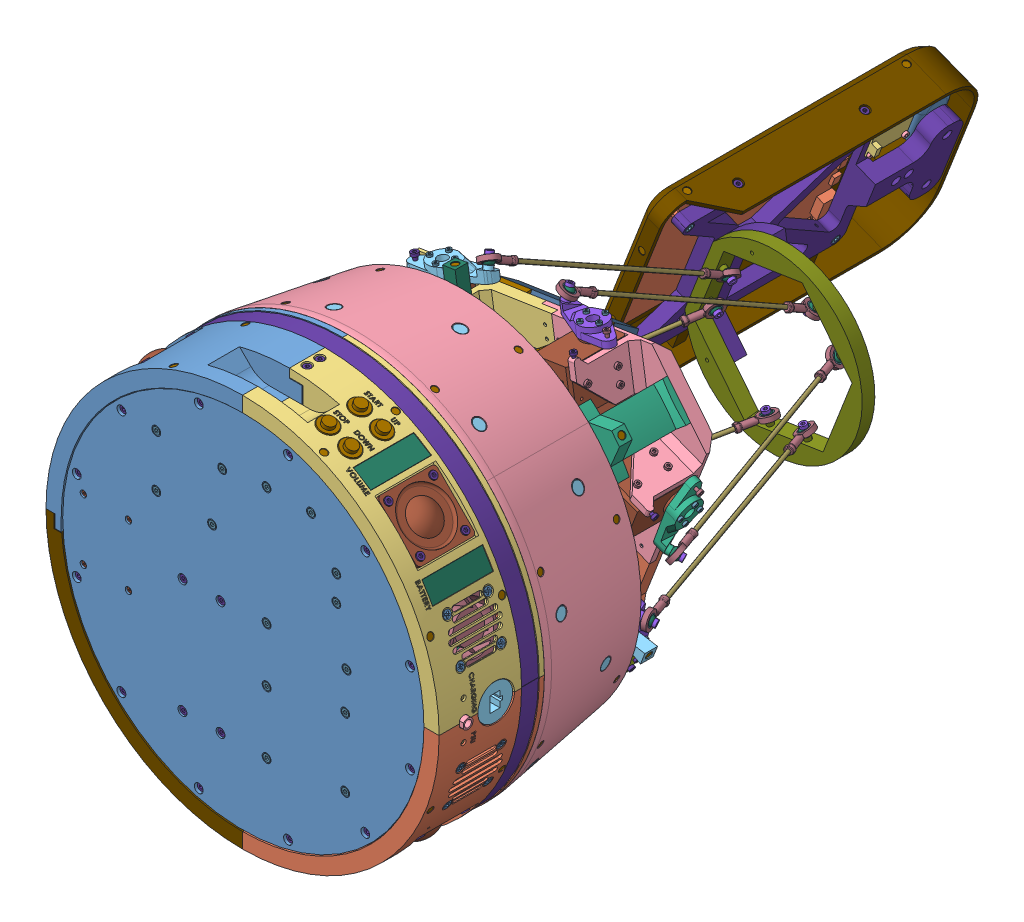
SolidWorks assembly robot orin, configuration Défaut. Lengths in mm.
Overall size (438.41 438.41 602.06).
668 component instances, 95 part files, 23 mates.
Components (placement in the parent):
- base-1: base [Défaut] at (-67.3784 29.2661 438.4062) size (438.41 438.41 173)
  - base disk-1: base disk [Défaut] at (36.9194 20.0613 317) size (285 285 66.55)
    - base disk-1: base disk [Défaut] at (-39.9498 -9.3034 266.18) size (285 285 6.35)
    - Adafruit MAX9744-1: Adafruit MAX9744 [Défaut] at (-148.3839 -9.3034 256.18) x (0 1 0) z (0 0 -1) size (56.74 43.64 13.6)
    - Adafruit MAX9744-2: Adafruit MAX9744 [Défaut] at (-148.3839 -9.3034 239.58) x (0 1 0) z (0 0 -1) size (56.74 43.64 13.6)
    - Battery charger RRC-PMM240-1: Battery charger RRC-PMM240 [Défaut] at (-52.8471 67.1868 256.18) x (0 -1 0) z (0 0 -1) size (57 70 12)
    - battery holder-1: battery holder [Défaut] at (-92.9498 0.6966 266.18) x (0 -1 0) z (1 0 0) size (115 36.2 40)
    - Battery RRC2054-2-1: Battery RRC2054-2 [Défaut] at (-82.3791 -10.7125 233.18) x (0 1 0) z (0 0 1) size (151 78 23)
    - ground loop noise isolator-1: ground loop noise isolator [Défaut] at (-105.1098 -100.3034 233.18) x (0 -1 0) z (1 0 0) size (20 20 60)
    - ground loop noise isolator-2: ground loop noise isolator [Défaut] at (-45.1098 -80.3034 233.18) x (0 0 1) z (-1 0 0) size (20 20 60)
    - psu control-1: psu control [Défaut] at (-25.1498 95.1966 256.18) x (0 -1 0) z (0 0 -1) size (100 70 16.5)
    - buck boost-1: buck boost [Défaut] at (-25.6498 -27.3034 256.18) x (0 -1 0) z (0 0 -1) size (80 70 23.6)
    - buck boost-2: buck boost [Défaut] at (-25.6498 -27.3034 229.58) x (0 -1 0) z (0 0 -1) size (80 70 23.6)
    - 732-12936-ND-1: 732-12936-ND [Défaut] at (-166.1639 14.8266 254.58) x (-0.923728 -0.383049 0) z (0 0 -1) size (4.6 4.17 20)
    - 732-12936-ND-2: 732-12936-ND [Défaut] at (-166.1639 -33.4334 254.58) x (-0.923728 -0.383049 0) z (0 0 -1) size (4.6 4.17 20)
    - 732-12936-ND-3: 732-12936-ND [Défaut] at (-130.6039 -33.4334 254.58) x (-0.923728 -0.383049 0) z (0 0 -1) size (4.6 4.17 20)
    - 732-12936-ND-4: 732-12936-ND [Défaut] at (-130.6039 14.8266 254.58) x (-0.923728 -0.383049 0) z (0 0 -1) size (4.6 4.17 20)
    - 732-12918-ND-1: 732-12918-ND [Défaut] at (-166.1639 14.8266 266.18) x (-0.923728 -0.383049 0) z (0 0 -1) size (4.6 4.17 15)
    - 732-12918-ND-2: 732-12918-ND [Défaut] at (-130.6039 14.8266 266.18) x (-0.923728 -0.383049 0) z (0 0 -1) size (4.6 4.17 15)
    - 732-12918-ND-3: 732-12918-ND [Défaut] at (-130.6039 -33.4334 266.18) x (-0.923728 -0.383049 0) z (0 0 -1) size (4.6 4.17 15)
    - 732-12918-ND-4: 732-12918-ND [Défaut] at (-166.1639 -33.4334 266.18) x (-0.923728 -0.383049 0) z (0 0 -1) size (4.6 4.17 15)
    - M2x8mm socket-6: M2x8mm socket [Défaut] at (-166.1639 -33.4334 262.03) x (-1 0 0) z (0 0 1) size (3.8 3.8 9.6)
    - M2x8mm socket-5: M2x8mm socket [Défaut] at (-130.6039 -33.4334 262.03) x (-1 0 0) z (0 0 1) size (3.8 3.8 9.6)
    - M2x8mm socket-3: M2x8mm socket [Défaut] at (-166.1639 14.8266 262.03) size (3.8 3.8 9.6)
    - M2x8mm socket-4: M2x8mm socket [Défaut] at (-130.6039 14.8266 262.03) x (-1 0 0) z (0 0 1) size (3.8 3.8 9.6)
    - M2 nut-1: M2 nut [Défaut] at (-166.1639 14.8266 237.98) x (-0.923728 -0.383049 0) z (0 0 -1) size (4.62 4 1.6)
    - M2 nut-2: M2 nut [Défaut] at (-166.1639 -33.4334 237.98) x (-0.923728 -0.383049 0) z (0 0 -1) size (4.62 4 1.6)
    - M2 nut-3: M2 nut [Défaut] at (-130.6039 -33.4334 237.98) x (-0.923728 -0.383049 0) z (0 0 -1) size (4.62 4 1.6)
    - M2 nut-4: M2 nut [Défaut] at (-130.6039 14.8266 237.98) x (-0.923728 -0.383049 0) z (0 0 -1) size (4.62 4 1.6)
    - 36-24337-ND-1: 36-24337-ND [Défaut] at (-108.6498 86.6966 266.18) x (-0.923728 -0.383049 0) z (0 0 -1) size (5.77 5 18)
    - 36-24337-ND-2: 36-24337-ND [Défaut] at (-108.6498 45.6966 266.18) x (-0.923728 -0.383049 0) z (0 0 -1) size (5.77 5 18)
    - 36-24337-ND-3: 36-24337-ND [Défaut] at (-64.6498 44.6966 266.18) x (-0.923728 -0.383049 0) z (0 0 -1) size (5.77 5 18)
    - 36-24337-ND-4: 36-24337-ND [Défaut] at (-56.6498 86.6966 266.18) x (-0.923728 -0.383049 0) z (0 0 -1) size (5.77 5 18)
    - M3x5mm socket-1: M3x5mm socket [Défaut] at (-108.6498 86.6966 264.53) x (-1 0 0) z (0 0 1) size (5.5 5.5 8)
    - M3x5mm socket-2: M3x5mm socket [Défaut] at (-108.6498 45.6966 264.53) x (-1 0 0) z (0 0 1) size (5.5 5.5 8)
    - M3x5mm socket-3: M3x5mm socket [Défaut] at (-64.6498 44.6966 264.53) x (-1 0 0) z (0 0 1) size (5.5 5.5 8)
    - M3x5mm socket-4: M3x5mm socket [Défaut] at (-56.6498 86.6966 264.53) x (-1 0 0) z (0 0 1) size (5.5 5.5 8)
    - M3 nut-1: M3 nut [Défaut] at (-108.6498 86.6966 254.18) x (-0.923728 -0.383049 0) z (0 0 -1) size (6.35 5.5 2.4)
    - M3 nut-2: M3 nut [Défaut] at (-108.6498 45.6966 254.18) x (-0.923728 -0.383049 0) z (0 0 -1) size (6.35 5.5 2.4)
    - M3 nut-3: M3 nut [Défaut] at (-64.6498 44.6966 254.18) x (-0.923728 -0.383049 0) z (0 0 -1) size (6.35 5.5 2.4)
    - M3 nut-4: M3 nut [Défaut] at (-56.6498 86.6966 254.18) x (-0.923728 -0.383049 0) z (0 0 -1) size (6.35 5.5 2.4)
    - 36-24337-ND-5: 36-24337-ND [Défaut] at (-21.6498 91.6966 266.18) x (-0.923728 -0.383049 0) z (0 0 -1) size (5.77 5 18)
    - 36-24337-ND-6: 36-24337-ND [Défaut] at (-21.6498 -1.3034 266.18) x (1 0 0) z (0 0 -1) size (5.77 5 18)
    - 36-24337-ND-7: 36-24337-ND [Défaut] at (13.3502 91.6966 266.18) x (0.923728 0.383049 0) z (0 0 -1) size (5.77 5 18)
    - 36-24337-ND-8: 36-24337-ND [Défaut] at (41.3502 -1.3034 266.18) x (-1 0 0) z (0 0 -1) size (5.77 5 18)
    - M3 nut-5: M3 nut [Défaut] at (-21.6498 91.6966 256.98) x (-1 0 0) z (0 0 -1) size (6.35 5.5 2.4)
    - M3 nut-6: M3 nut [Défaut] at (13.3502 91.6966 252.18) x (-1 0 0) z (0 0 1) size (6.35 5.5 2.4)
    - M3 nut-7: M3 nut [Défaut] at (-21.6498 -1.3034 252.18) x (-1 0 0) z (0 0 1) size (6.35 5.5 2.4)
    - M3 nut-8: M3 nut [Défaut] at (41.3502 -1.3034 252.18) size (6.35 5.5 2.4)
    - 36-24337-ND-9: 36-24337-ND [Défaut] at (-21.6498 -44.3034 266.18) x (-0.923728 -0.383049 0) z (0 0 -1) size (5.77 5 18)
    - 36-24337-ND-10: 36-24337-ND [Défaut] at (-21.6498 -93.3034 266.18) x (-0.923728 -0.383049 0) z (0 0 -1) size (5.77 5 18)
    - 36-24337-ND-11: 36-24337-ND [Défaut] at (40.3502 -85.3034 266.18) x (-0.923728 -0.383049 0) z (0 0 -1) size (5.77 5 18)
    - 36-24337-ND-12: 36-24337-ND [Défaut] at (40.3502 -31.3034 266.18) x (-0.923728 -0.383049 0) z (0 0 -1) size (5.77 5 18)
    - 36-24342-ND-1: 36-24342-ND [Défaut] at (-21.6498 -44.3034 254.58) x (1 0 0) z (0 0 -1) size (5.77 5 33)
    - 36-24342-ND-2: 36-24342-ND [Défaut] at (-21.6498 -93.3034 254.58) x (1 0 0) z (0 0 -1) size (5.77 5 33)
    - 36-24342-ND-3: 36-24342-ND [Défaut] at (40.3502 -31.3034 254.58) x (1 0 0) z (0 0 -1) size (5.77 5 33)
    - 36-24342-ND-4: 36-24342-ND [Défaut] at (40.3502 -85.3034 254.58) x (1 0 0) z (0 0 -1) size (5.77 5 33)
    - M3 nut-9: M3 nut [Défaut] at (40.3502 -31.3034 227.98) x (-1 0 0) z (0 0 -1) size (6.35 5.5 2.4)
    - M3 nut-10: M3 nut [Défaut] at (-21.6498 -44.3034 227.98) x (-1 0 0) z (0 0 -1) size (6.35 5.5 2.4)
    - M3 nut-11: M3 nut [Défaut] at (-21.6498 -93.3034 225.58) size (6.35 5.5 2.4)
    - M3 nut-12: M3 nut [Défaut] at (40.3502 -85.3034 227.98) x (-1 0 0) z (0 0 -1) size (6.35 5.5 2.4)
    - 36-24337-ND-13: 36-24337-ND [Défaut] at (33.3502 60.1966 266.18) x (-0.923728 -0.383049 0) z (0 0 -1) size (5.77 5 18)
    - 36-24337-ND-14: 36-24337-ND [Défaut] at (33.3502 40.1966 266.18) x (-0.923728 -0.383049 0) z (0 0 -1) size (5.77 5 18)
    - M3 nut-13: M3 nut [Défaut] at (33.3502 60.1966 252.18) size (6.35 5.5 2.4)
    - M3 nut-14: M3 nut [Défaut] at (33.3502 40.1966 252.18) size (6.35 5.5 2.4)
    - M3x8mm plastic-1: M3x8mm plastic [Défaut] at (-57.9498 -4.3034 261.53) size (5.5 5.5 10.3)
    - M3x8mm plastic-2: M3x8mm plastic [Défaut] at (-57.9498 -94.3034 261.53) size (5.5 5.5 10.3)
    - M3x8mm plastic-3: M3x8mm plastic [Défaut] at (-87.9498 -94.3034 261.53) size (5.5 5.5 10.3)
    - M3x8mm plastic-4: M3x8mm plastic [Défaut] at (-87.9498 -4.3034 261.53) size (5.5 5.5 10.3)
    - M3x5mm socket-5: M3x5mm socket [Défaut] at (-21.6498 91.6966 264.53) size (5.5 5.5 8)
    - M3x5mm socket-6: M3x5mm socket [Défaut] at (13.3502 91.6966 264.53) size (5.5 5.5 8)
    - M3x5mm socket-7: M3x5mm socket [Défaut] at (33.3502 60.1966 264.53) size (5.5 5.5 8)
    - M3x5mm socket-8: M3x5mm socket [Défaut] at (33.3502 40.1966 264.53) size (5.5 5.5 8)
    - M3x5mm socket-9: M3x5mm socket [Défaut] at (-21.6498 -1.3034 264.53) size (5.5 5.5 8)
    - M3x5mm socket-10: M3x5mm socket [Défaut] at (-21.6498 -44.3034 264.53) size (5.5 5.5 8)
    - M3x5mm socket-11: M3x5mm socket [Défaut] at (-21.6498 -93.3034 264.53) size (5.5 5.5 8)
    - M3x5mm socket-12: M3x5mm socket [Défaut] at (40.3502 -85.3034 264.53) size (5.5 5.5 8)
    - M3x5mm socket-13: M3x5mm socket [Défaut] at (40.3502 -31.3034 264.53) size (5.5 5.5 8)
    - M3x5mm socket-14: M3x5mm socket [Défaut] at (41.3502 -1.3034 264.53) size (5.5 5.5 8)
  - base audio-1: base audio [Défaut] at (-77.1238 -92.9542 353.528) x (0 1 0) z (0 0 1) size (420.86 420.86 86)
    - base audio front left-1: base audio front left [Défaut] at (103.7122 -74.0934 171.652) size (155 165 86)
    - base audio front right-1: base audio front right [Défaut] at (103.7122 -74.0934 171.652) x (0 -1 0) z (0 0 1) size (165 165 86)
    - base audio back left-1: base audio back left [Défaut] at (103.7122 -74.0934 171.652) x (0 1 0) z (0 0 1) size (155 156 86)
    - base audio back right-1: base audio back right [Défaut] at (103.7122 -74.0934 171.652) x (-1 0 0) z (0 0 1) size (156 155 86)
    - SC2073-ND-1: SC2073-ND [Défaut] at (103.7122 -222.6934 217.152) x (1 0 0) z (0 -1 0) size (11.94 11.94 36.36)
    - RJ45 connector-1: RJ45 connector [Défaut] at (103.7122 -228.0934 191.652) x (1 0 0) z (0 1 0) size (27.9 27.9 35.9)
    - Micro USB B (Adafruit 4217)-1: Micro USB B (Adafruit 4217) [Défaut] at (-6.0335 -126.2291 211.652) x (-0.429101 0.903257 0) z (0 0 1) size (28 33.5 28)
    - Micro USB B nut (Adafruit 4217)-1: Micro USB B nut (Adafruit 4217) [Défaut] at (-28.6149 -136.9566 211.652) x (0.18262 -0.384415 -0.904917) z (0.903257 0.429101 0) size (30.02 30.02 8)
    - switch-1: switch [Défaut] at (-36.2542 -140.9179 186.027) x (0.429101 -0.903257 0) z (0.903257 0.429101 0) size (20.75 14.7 24.67)
    - button-1: button [Défaut] at (254.7907 -122.0257 191.152) x (0.197389 0.622151 -0.757605) z (-0.953177 0.302412 0) size (14 14 27.8)
    - button-2: button [Défaut] at (247.8231 -140.0803 191.152) x (0.179537 0.392097 -0.902234) z (-0.909218 0.416321 0) size (14 14 27.8)
    - button-3: button [Défaut] at (254.7907 -122.0257 216.152) x (0.197389 0.622151 -0.757605) z (-0.953177 0.302412 0) size (14 14 27.8)
    - button-4: button [Défaut] at (247.8231 -140.0803 216.152) x (0.179537 0.392097 -0.902234) z (-0.909218 0.416321 0) size (14 14 27.8)
    - button nut-1: button nut [Défaut] at (247.1653 -119.6064 191.152) x (0.099317 0.313039 0.944533) z (-0.953177 0.302412 0) size (16 16 5)
    - button nut-2: button nut [Défaut] at (247.1653 -119.6064 216.152) x (0.099317 0.313039 0.944533) z (-0.953177 0.302412 0) size (16 16 5)
    - button nut-3: button nut [Défaut] at (240.5494 -136.7497 216.152) x (0.182325 0.398185 0.899003) z (-0.909218 0.416321 0) size (16 16 5)
    - button nut-4: button nut [Défaut] at (240.5494 -136.7497 191.152) x (0.179537 0.392097 -0.902234) z (-0.909218 0.416321 0) size (16 16 5) (hidden)
    - Dayton Audio DMA45-8-1: Dayton Audio DMA45-8 [Défaut] at (209.7782 -180.1594 199.652) x (0.707107 0.707107 0) z (0.707107 -0.707107 0) size (46 46 32.1)
    - Dayton Audio DMA45-8-2: Dayton Audio DMA45-8 [Défaut] at (209.7782 31.9727 199.652) x (-0.707107 0.707107 0) z (0.707107 0.707107 0) size (46 46 32.1)
    - Dayton Audio DMA45-8-3: Dayton Audio DMA45-8 [Défaut] at (-2.3539 31.9727 199.652) x (-0.707107 -0.707107 0) z (-0.707107 0.707107 0) size (46 46 32.1)
    - Dayton Audio DMA45-8-4: Dayton Audio DMA45-8 [Défaut] at (-2.3539 -180.1594 199.652) x (0.707107 -0.707107 0) z (-0.707107 -0.707107 0) size (46 46 32.1)
    - LED 5mm-1: LED 5mm [Défaut] at (88.5685 -227.8494 216.652) x (-0.876134 0.086292 -0.474281) z (0.098017 0.995185 0) size (5.5 5.5 18.7)
    - LED 5mm-2: LED 5mm [Défaut] at (118.8558 -227.8494 216.652) x (-0.780695 -0.076892 -0.620163) z (-0.098017 0.995185 0) size (5.5 5.5 18.7)
    - Noctua NF-A4X20-1: Noctua NF-A4X20 [Défaut] at (61.6633 -197.158 199.652) x (0.946287 -0.323328 0) z (-0.323328 -0.946287 0) size (39.9 39.9 19.95)
    - Noctua NF-A4X20-2: Noctua NF-A4X20 [Défaut] at (145.761 -197.158 199.652) x (0.946287 0.323328 0) z (0.323328 -0.946287 0) size (39.9 39.9 19.95)
    - LED level-1: LED level [Défaut] at (232.9084 -146.5387 181.6389) x (0.524024 0.851704 0) z (0.851704 -0.524024 0) size (12 34.5 2)
    - LED level-2: LED level [Défaut] at (185.0786 -197.8654 181.6389) x (0.857177 0.515023 0) z (0.515023 -0.857177 0) size (12 34.5 2)
    - LED level diffuser-1: LED level diffuser [Défaut] at (240.4553 -143.8142 199.2629) x (0.524024 0.851704 0) z (0.851704 -0.524024 0) size (16 47.5 1.59)
    - LED level diffuser-2: LED level diffuser [Défaut] at (193.0327 -198.9193 199.2629) x (0.857177 0.515023 0) z (0.515023 -0.857177 0) size (16 47.5 1.59)
    - LED strip-1: LED strip [Défaut] at (103.7122 -74.0934 159.902) x (0.707107 -0.707107 0) z (0 0 1) size (297.3 297.88 9.5)
    - LED strip diffuser (round)-1: LED strip diffuser (round) [Défaut] at (103.7122 -74.0934 157.902) x (0.000809 -1 0) z (0 0 1) size (309.17 309.17 13.5)
    - light sensor-1: light sensor [Défaut] at (228.5122 -87.4674 238.7403) x (0 0 -1) z (1 0 0) size (7.62 10.16 4.2)
    - light sensor-2: light sensor [Défaut] at (-21.0878 -87.4674 196.0637) x (0 0 1) z (-1 0 0) size (7.62 10.16 4.2)
    - light sensor-3: light sensor [Défaut] at (29.9331 -198.7828 198.0637) x (0 0 1) z (-0.537899 -0.843009 0) size (7.62 10.16 4.2)
    - light sensor-4: light sensor [Défaut] at (109.4763 70.6739 198.0637) x (0 0 1) z (0.073377 0.997304 0) size (7.62 10.16 4.2)
    - M3x8mm plastic-1: M3x8mm plastic [Défaut] at (98.7122 69.9066 183.652) x (1 0 0) z (0 1 0) size (5.5 5.5 10.3)
    - M3x8mm plastic-2: M3x8mm plastic [Défaut] at (98.7122 69.9066 213.652) x (1 0 0) z (0 1 0) size (5.5 5.5 10.3)
    - M3x8mm plastic-3: M3x8mm plastic [Défaut] at (-40.2878 -79.0934 180.652) x (0 0 1) z (-1 0 0) size (5.5 5.5 10.3)
    - M3x8mm plastic-4: M3x8mm plastic [Défaut] at (-40.2878 -79.0934 190.652) x (0 0 1) z (-1 0 0) size (5.5 5.5 10.3)
    - M3x8mm plastic-5: M3x8mm plastic [Défaut] at (247.7122 -79.0934 180.652) x (0 0 -1) z (1 0 0) size (5.5 5.5 10.3)
    - M3x8mm plastic-6: M3x8mm plastic [Défaut] at (247.7122 -79.0934 190.652) x (0 0 -1) z (1 0 0) size (5.5 5.5 10.3)
    - M3x8mm plastic-8: M3x8mm plastic [Défaut] at (192.6308 -188.1143 181.902) x (0.5 0.5 -0.707107) z (0.707107 -0.707107 0) size (5.5 5.5 10.3)
    - M3x8mm plastic-14: M3x8mm plastic [Défaut] at (-10.3088 -163.012 181.902) x (0.5 -0.5 -0.707107) z (-0.707107 -0.707107 0) size (5.5 5.5 10.3)
    - M3x8mm plastic-13: M3x8mm plastic [Défaut] at (14.7935 39.9276 181.902) x (-0.5 -0.5 -0.707107) z (-0.707107 0.707107 0) size (5.5 5.5 10.3)
    - M3x8mm plastic-12: M3x8mm plastic [Défaut] at (217.7331 14.8253 181.902) x (-0.5 0.5 -0.707107) z (0.707107 0.707107 0) size (5.5 5.5 10.3)
    - M3x8mm plastic-9: M3x8mm plastic [Défaut] at (217.7331 -163.012 217.402) x (0.5 0.5 -0.707107) z (0.707107 -0.707107 0) size (5.5 5.5 10.3)
    - M3x8mm plastic-17: M3x8mm plastic [Défaut] at (14.7935 -188.1143 217.402) x (0.5 -0.5 -0.707107) z (-0.707107 -0.707107 0) size (5.5 5.5 10.3)
    - M3x8mm plastic-16: M3x8mm plastic [Défaut] at (-10.3088 14.8253 217.402) x (-0.5 -0.5 -0.707107) z (-0.707107 0.707107 0) size (5.5 5.5 10.3)
    - M3x8mm plastic-15: M3x8mm plastic [Défaut] at (192.6308 39.9276 217.402) x (-0.5 0.5 -0.707107) z (0.707107 0.707107 0) size (5.5 5.5 10.3)
    - M3x8mm plastic-10: M3x8mm plastic [Défaut] at (192.6308 -188.1143 217.402) x (0.5 0.5 -0.707107) z (0.707107 -0.707107 0) size (5.5 5.5 10.3)
    - M3x8mm plastic-20: M3x8mm plastic [Défaut] at (-10.3088 -163.012 217.402) x (0.5 -0.5 -0.707107) z (-0.707107 -0.707107 0) size (5.5 5.5 10.3)
    - M3x8mm plastic-19: M3x8mm plastic [Défaut] at (14.7935 39.9276 217.402) x (-0.5 -0.5 -0.707107) z (-0.707107 0.707107 0) size (5.5 5.5 10.3)
    - M3x8mm plastic-18: M3x8mm plastic [Défaut] at (217.7331 14.8253 217.402) x (-0.5 0.5 -0.707107) z (0.707107 0.707107 0) size (5.5 5.5 10.3)
    - M3x8mm plastic-11: M3x8mm plastic [Défaut] at (217.7331 -163.012 181.902) x (0.5 0.5 -0.707107) z (0.707107 -0.707107 0) size (5.5 5.5 10.3)
    - M3x8mm plastic-23: M3x8mm plastic [Défaut] at (14.7935 -188.1143 181.902) x (0.5 -0.5 -0.707107) z (-0.707107 -0.707107 0) size (5.5 5.5 10.3)
    - M3x8mm plastic-22: M3x8mm plastic [Défaut] at (-10.3088 14.8253 181.902) x (-0.5 -0.5 -0.707107) z (-0.707107 0.707107 0) size (5.5 5.5 10.3)
    - M3x8mm plastic-21: M3x8mm plastic [Défaut] at (192.6308 39.9276 181.902) x (-0.5 0.5 -0.707107) z (0.707107 0.707107 0) size (5.5 5.5 10.3)
    - fan screw-1: fan screw [Défaut] at (165.5737 -205.6586 183.652) x (0.879667 0.300565 -0.368573) z (0.323328 -0.946287 0) size (6.3 6.3 9.5)
    - fan screw-2: fan screw [Défaut] at (165.5737 -205.6586 215.652) x (0.879667 0.300565 -0.368573) z (0.323328 -0.946287 0) size (6.3 6.3 9.5)
    - fan screw-3: fan screw [Défaut] at (135.2925 -216.0051 215.652) x (-0.927498 -0.316908 -0.198283) z (0.323328 -0.946287 0) size (6.3 6.3 9.5)
    - fan screw-4: fan screw [Défaut] at (135.2925 -216.0051 183.652) x (0.879667 0.300565 -0.368573) z (0.323328 -0.946287 0) size (6.3 6.3 9.5)
    - fan screw-5: fan screw [Défaut] at (72.1318 -216.0051 183.652) x (0.879667 -0.300565 0.368573) z (-0.323328 -0.946287 0) size (6.3 6.3 9.5)
    - fan screw-6: fan screw [Défaut] at (72.1318 -216.0051 215.652) x (0.879667 -0.300565 0.368573) z (-0.323328 -0.946287 0) size (6.3 6.3 9.5)
    - fan screw-7: fan screw [Défaut] at (41.8506 -205.6586 215.652) x (0.879667 -0.300565 0.368573) z (-0.323328 -0.946287 0) size (6.3 6.3 9.5)
    - fan screw-8: fan screw [Défaut] at (41.8506 -205.6586 183.652) x (0.879667 -0.300565 0.368573) z (-0.323328 -0.946287 0) size (6.3 6.3 9.5)
    - dewel pin 0.125in 0.5in-1: dewel pin 0.125in 0.5in [Défaut] at (111.2122 -212.8434 155.652) x (0 0 1) z (-1 0 0) size (3.17 3.17 12.7)
    - dewel pin 0.125in 0.5in-2: dewel pin 0.125in 0.5in [Défaut] at (111.2122 -223.0934 228.6844) x (0 0 1) z (-1 0 0) size (3.17 3.17 12.7)
    - M2x5mm plastic-1: M2x5mm plastic [Défaut] at (233.5122 -79.5934 217.402) x (0 0.924225 0.381849) z (-1 0 0) size (3.35 3.35 6.6)
    - M2x5mm plastic-2: M2x5mm plastic [Défaut] at (-26.0878 -79.5934 217.402) x (0 0.5 -0.866025) z (1 0 0) size (3.35 3.35 6.6)
    - M2x5mm plastic-3: M2x5mm plastic [Défaut] at (20.6058 -198.7624 219.402) x (-0.826053 0.527081 -0.199554) z (0.537899 0.843009 0) size (3.35 3.35 6.6)
    - M2x5mm plastic-4: M2x5mm plastic [Défaut] at (117.696 75.0827 219.402) x (0.994616 -0.073179 0.073377) z (-0.073377 -0.997304 0) size (3.35 3.35 6.6)
  - base mic-1: base mic [Défaut] at (-78.91 184.7021 463.131) x (-0.707107 -0.707107 0) z (0.707107 -0.707107 0) size (310 92.85 310)
    - base mic-1: base mic [Défaut] at (69.3421 -41.049 176.652) size (155 90 160)
    - 8SoundsUSB Mic-1: 8SoundsUSB Mic [Défaut] at (30.5719 -34.8926 320.3049) x (0.980785 0 0.19509) z (-0.192688 0.156434 0.96871) size (25.4 23.4 21.48)
    - 8SoundsUSB Mic-2: 8SoundsUSB Mic [Défaut] at (-17.8103 6.4759 289.0854) x (0.83147 0 0.55557) z (-0.54873 0.156434 0.821233) size (25.4 23.4 21.48)
    - 8SoundsUSB Mic-3: 8SoundsUSB Mic [Défaut] at (-71.7864 6.4759 194.5283) x (0.19509 0 0.980785) z (-0.96871 0.156434 0.192688) size (25.4 23.4 21.48)
    - 8SoundsUSB Mic-4: 8SoundsUSB Mic [Défaut] at (-59.6505 -34.8926 250.8153) x (0.55557 0 0.83147) z (-0.821233 0.156434 0.54873) size (25.4 23.4 21.48)
    - 16SoundsUSB-1: 16SoundsUSB [Défaut] at (69.3421 -36.049 176.6521) x (1 0 0) z (0 -1 0) size (165.86 165.78 26.13)
    - M3x5mm plastic-1: M3x5mm plastic [Défaut] at (49.8528 -16.3964 325.89) x (-0.186611 0.963352 -0.192688) z (0.192688 -0.156434 -0.96871) size (5.5 5.5 7.3)
    - M3x5mm plastic-2: M3x5mm plastic [Défaut] at (30.2371 -16.3964 321.9882) x (-0.186611 0.963352 -0.192688) z (0.192688 -0.156434 -0.96871) size (5.5 5.5 7.3)
    - M3x5mm plastic-3: M3x5mm plastic [Défaut] at (49.3034 -34.1748 328.6517) x (-0.186611 0.963352 -0.192688) z (0.192688 -0.156434 -0.96871) size (5.5 5.5 7.3)
    - M3x5mm plastic-4: M3x5mm plastic [Défaut] at (29.6877 -34.1748 324.7499) x (-0.186611 0.963352 -0.192688) z (0.192688 -0.156434 -0.96871) size (5.5 5.5 7.3)
    - M3x5mm plastic-5: M3x5mm plastic [Défaut] at (-2.1344 24.9721 301.6238) x (-0.684341 0.480179 -0.54873) z (0.54873 -0.156434 -0.821233) size (5.5 5.5 7.3)
    - M3x5mm plastic-6: M3x5mm plastic [Défaut] at (-18.7638 24.9721 290.5124) x (-0.684341 0.480179 -0.54873) z (0.54873 -0.156434 -0.821233) size (5.5 5.5 7.3)
    - M3x5mm plastic-7: M3x5mm plastic [Défaut] at (-3.6988 7.1937 303.965) x (-0.684341 0.480179 -0.54873) z (0.54873 -0.156434 -0.821233) size (5.5 5.5 7.3)
    - M3x5mm plastic-8: M3x5mm plastic [Défaut] at (-20.3282 7.1937 292.8536) x (-0.684341 0.480179 -0.54873) z (0.54873 -0.156434 -0.821233) size (5.5 5.5 7.3)
    - M3x5mm plastic-9: M3x5mm plastic [Défaut] at (-49.9661 -16.3964 268.3981) x (-0.494502 0.284684 -0.821233) z (0.821233 -0.156434 -0.54873) size (5.5 5.5 7.3)
    - M3x5mm plastic-10: M3x5mm plastic [Défaut] at (-61.0775 -16.3964 251.7687) x (-0.494502 0.284684 -0.821233) z (0.821233 -0.156434 -0.54873) size (5.5 5.5 7.3)
    - M3x5mm plastic-11: M3x5mm plastic [Défaut] at (-63.4188 -34.1748 253.3331) x (-0.494502 0.284684 -0.821233) z (0.821233 -0.156434 -0.54873) size (5.5 5.5 7.3)
    - M3x5mm plastic-12: M3x5mm plastic [Défaut] at (-52.3074 -34.1748 269.9625) x (-0.494502 0.284684 -0.821233) z (0.821233 -0.156434 -0.54873) size (5.5 5.5 7.3)
    - M3x5mm plastic-13: M3x5mm plastic [Défaut] at (-72.3295 7.1937 215.0282) x (-0.225994 -0.876896 -0.424241) z (0.96871 -0.156434 -0.192688) size (5.5 5.5 7.3)
    - M3x5mm plastic-14: M3x5mm plastic [Défaut] at (-69.5678 24.9721 214.4788) x (-0.162376 0.187709 -0.96871) z (0.96871 -0.156434 -0.192688) size (5.5 5.5 7.3)
    - M3x5mm plastic-15: M3x5mm plastic [Défaut] at (-73.4696 24.9721 194.8631) x (-0.162376 0.187709 -0.96871) z (0.96871 -0.156434 -0.192688) size (5.5 5.5 7.3)
    - M3x5mm plastic-16: M3x5mm plastic [Défaut] at (-76.2313 7.1937 195.4125) x (-0.162376 0.187709 -0.96871) z (0.96871 -0.156434 -0.192688) size (5.5 5.5 7.3)
    - M3x8mm plastic-1: M3x8mm plastic [Défaut] at (15.9671 -42.4056 230.027) x (1 0 0) z (0 1 0) size (5.5 5.5 10.3)
    - M3x8mm plastic-2: M3x8mm plastic [Défaut] at (122.7171 -42.4056 230.027) x (1 0 0) z (0 1 0) size (5.5 5.5 10.3)
    - M3x8mm plastic-3: M3x8mm plastic [Défaut] at (15.9671 -42.4056 123.277) x (-0.837169 0 -0.546944) z (0 1 0) size (5.5 5.5 10.3)
    - M3x8mm plastic-4: M3x8mm plastic [Défaut] at (122.7171 -42.4056 123.277) x (-0.837169 0 -0.546944) z (0 1 0) size (5.5 5.5 10.3)
    - M3x5mm plastic-17: M3x5mm plastic [Défaut] at (-75.994 -16.3964 137.547) x (0.192688 0.963352 -0.186611) z (0.96871 -0.156434 0.192688) size (5.5 5.5 7.3)
    - M3x5mm plastic-18: M3x5mm plastic [Défaut] at (108.4472 -16.3964 31.3159) x (0.186611 0.963352 0.192688) z (-0.192688 -0.156434 0.96871) size (5.5 5.5 7.3)
    - M3x5mm plastic-19: M3x5mm plastic [Défaut] at (214.6783 -16.3964 215.7571) x (-0.192688 0.963352 0.186611) z (-0.96871 -0.156434 -0.192688) size (5.5 5.5 7.3)
    - M3x5mm plastic-20: M3x5mm plastic [Défaut] at (-82.6575 -34.1748 156.6133) x (0.192688 0.963352 -0.186611) z (0.96871 -0.156434 0.192688) size (5.5 5.5 7.3)
    - M3x5mm plastic-21: M3x5mm plastic [Défaut] at (89.3808 -34.1748 24.6524) x (0.186611 0.963352 0.192688) z (-0.192688 -0.156434 0.96871) size (5.5 5.5 7.3)
    - M3x5mm plastic-22: M3x5mm plastic [Défaut] at (221.3418 -34.1748 196.6907) x (-0.192688 0.963352 0.186611) z (-0.96871 -0.156434 -0.192688) size (5.5 5.5 7.3)
    - M3x5mm plastic-23: M3x5mm plastic [Défaut] at (-78.7557 -34.1748 136.9976) x (0.192688 0.963352 -0.186611) z (0.96871 -0.156434 0.192688) size (5.5 5.5 7.3)
    - M3x5mm plastic-24: M3x5mm plastic [Défaut] at (108.9965 -34.1748 28.5542) x (0.186611 0.963352 0.192688) z (-0.192688 -0.156434 0.96871) size (5.5 5.5 7.3)
    - M3x5mm plastic-25: M3x5mm plastic [Défaut] at (217.44 -34.1748 216.3064) x (-0.192688 0.963352 0.186611) z (-0.96871 -0.156434 -0.192688) size (5.5 5.5 7.3)
    - M3x5mm plastic-26: M3x5mm plastic [Défaut] at (-55.6296 24.9721 105.1755) x (0.54873 0.480179 -0.684341) z (0.821233 -0.156434 0.54873) size (5.5 5.5 7.3)
    - M3x5mm plastic-27: M3x5mm plastic [Défaut] at (140.8187 24.9721 51.6803) x (0.684341 0.480179 0.54873) z (-0.54873 -0.156434 0.821233) size (5.5 5.5 7.3)
    - M3x5mm plastic-28: M3x5mm plastic [Défaut] at (194.3139 24.9721 248.1286) x (-0.54873 0.480179 0.684341) z (-0.821233 -0.156434 -0.54873) size (5.5 5.5 7.3)
    - M3x5mm plastic-29: M3x5mm plastic [Défaut] at (-44.5182 24.9721 88.5461) x (0.54873 0.480179 -0.684341) z (0.821233 -0.156434 0.54873) size (5.5 5.5 7.3)
    - M3x5mm plastic-30: M3x5mm plastic [Défaut] at (157.4481 24.9721 62.7917) x (0.684341 0.480179 0.54873) z (-0.54873 -0.156434 0.821233) size (5.5 5.5 7.3)
    - M3x5mm plastic-31: M3x5mm plastic [Défaut] at (183.2025 24.9721 264.758) x (-0.54873 0.480179 0.684341) z (-0.821233 -0.156434 -0.54873) size (5.5 5.5 7.3)
    - M3x5mm plastic-32: M3x5mm plastic [Défaut] at (-57.9709 7.1937 103.6111) x (0.54873 0.480179 -0.684341) z (0.821233 -0.156434 0.54873) size (5.5 5.5 7.3)
    - M3x5mm plastic-33: M3x5mm plastic [Défaut] at (142.3831 7.1937 49.339) x (0.684341 0.480179 0.54873) z (-0.54873 -0.156434 0.821233) size (5.5 5.5 7.3)
    - M3x5mm plastic-34: M3x5mm plastic [Défaut] at (196.6551 7.1937 249.693) x (-0.54873 0.480179 0.684341) z (-0.821233 -0.156434 -0.54873) size (5.5 5.5 7.3)
    - M3x5mm plastic-35: M3x5mm plastic [Défaut] at (-46.8595 7.1937 86.9817) x (0.54873 0.480179 -0.684341) z (0.821233 -0.156434 0.54873) size (5.5 5.5 7.3)
    - M3x5mm plastic-36: M3x5mm plastic [Défaut] at (159.0125 7.1937 60.4504) x (0.684341 0.480179 0.54873) z (-0.54873 -0.156434 0.821233) size (5.5 5.5 7.3)
    - M3x5mm plastic-37: M3x5mm plastic [Défaut] at (185.5437 7.1937 266.3224) x (-0.54873 0.480179 0.684341) z (-0.821233 -0.156434 -0.54873) size (5.5 5.5 7.3)
    - M3x5mm plastic-38: M3x5mm plastic [Défaut] at (-22.404 -16.3964 57.3438) x (0.821233 0.284684 -0.494502) z (0.54873 -0.156434 0.821233) size (5.5 5.5 7.3)
    - M3x5mm plastic-39: M3x5mm plastic [Défaut] at (188.6504 -16.3964 84.9059) x (0.494502 0.284684 0.821233) z (-0.821233 -0.156434 0.54873) size (5.5 5.5 7.3)
    - M3x5mm plastic-40: M3x5mm plastic [Défaut] at (161.0882 -16.3964 295.9603) x (-0.821233 0.284684 0.494502) z (-0.54873 -0.156434 -0.821233) size (5.5 5.5 7.3)
    - M3x5mm plastic-41: M3x5mm plastic [Défaut] at (-5.7746 -16.3964 46.2324) x (0.821233 0.284684 -0.494502) z (0.54873 -0.156434 0.821233) size (5.5 5.5 7.3)
    - M3x5mm plastic-42: M3x5mm plastic [Défaut] at (199.7618 -16.3964 101.5353) x (0.494502 0.284684 0.821233) z (-0.821233 -0.156434 0.54873) size (5.5 5.5 7.3)
    - M3x5mm plastic-43: M3x5mm plastic [Défaut] at (144.4588 -16.3964 307.0717) x (-0.821233 0.284684 0.494502) z (-0.54873 -0.156434 -0.821233) size (5.5 5.5 7.3)
    - M3x5mm plastic-44: M3x5mm plastic [Défaut] at (-7.339 -34.1748 43.8911) x (0.821233 0.284684 -0.494502) z (0.54873 -0.156434 0.821233) size (5.5 5.5 7.3)
    - M3x5mm plastic-45: M3x5mm plastic [Défaut] at (202.103 -34.1748 99.9709) x (0.494502 0.284684 0.821233) z (-0.821233 -0.156434 0.54873) size (5.5 5.5 7.3)
    - M3x5mm plastic-46: M3x5mm plastic [Défaut] at (146.0232 -34.1748 309.4129) x (-0.821233 0.284684 0.494502) z (-0.54873 -0.156434 -0.821233) size (5.5 5.5 7.3)
    - M3x5mm plastic-47: M3x5mm plastic [Défaut] at (-23.9684 -34.1748 55.0025) x (0.821233 0.284684 -0.494502) z (0.54873 -0.156434 0.821233) size (5.5 5.5 7.3)
    - M3x5mm plastic-48: M3x5mm plastic [Défaut] at (190.9916 -34.1748 83.3415) x (0.494502 0.284684 0.821233) z (-0.821233 -0.156434 0.54873) size (5.5 5.5 7.3)
    - M3x5mm plastic-49: M3x5mm plastic [Défaut] at (162.6526 -34.1748 298.3015) x (-0.821233 0.284684 0.494502) z (-0.54873 -0.156434 -0.821233) size (5.5 5.5 7.3)
    - M3x5mm plastic-50: M3x5mm plastic [Défaut] at (30.966 7.1937 34.9804) x (0.424241 -0.876896 -0.225994) z (0.192688 -0.156434 0.96871) size (5.5 5.5 7.3)
    - M3x5mm plastic-51: M3x5mm plastic [Défaut] at (211.0138 7.1937 138.2759) x (0.225994 -0.876896 0.424241) z (-0.96871 -0.156434 0.192688) size (5.5 5.5 7.3)
    - M3x5mm plastic-52: M3x5mm plastic [Défaut] at (107.7183 7.1937 318.3237) x (-0.424241 -0.876896 0.225994) z (-0.192688 -0.156434 -0.96871) size (5.5 5.5 7.3)
    - M3x5mm plastic-53: M3x5mm plastic [Défaut] at (31.5153 24.9721 37.7421) x (0.96871 0.187709 -0.162376) z (0.192688 -0.156434 0.96871) size (5.5 5.5 7.3)
    - M3x5mm plastic-54: M3x5mm plastic [Défaut] at (208.252 24.9721 138.8252) x (0.162376 0.187709 0.96871) z (-0.96871 -0.156434 0.192688) size (5.5 5.5 7.3)
    - M3x5mm plastic-55: M3x5mm plastic [Défaut] at (107.1689 24.9721 315.5619) x (-0.96871 0.187709 0.162376) z (-0.192688 -0.156434 -0.96871) size (5.5 5.5 7.3)
    - M3x5mm plastic-56: M3x5mm plastic [Défaut] at (51.131 24.9721 33.8403) x (0.96871 0.187709 -0.162376) z (0.192688 -0.156434 0.96871) size (5.5 5.5 7.3)
    - M3x5mm plastic-57: M3x5mm plastic [Défaut] at (212.1539 24.9721 158.4409) x (0.162376 0.187709 0.96871) z (-0.96871 -0.156434 0.192688) size (5.5 5.5 7.3)
    - M3x5mm plastic-58: M3x5mm plastic [Défaut] at (87.5532 24.9721 319.4638) x (-0.96871 0.187709 0.162376) z (-0.192688 -0.156434 -0.96871) size (5.5 5.5 7.3)
    - M3x5mm plastic-59: M3x5mm plastic [Défaut] at (50.5817 7.1937 31.0786) x (0.96871 0.187709 -0.162376) z (0.192688 -0.156434 0.96871) size (5.5 5.5 7.3)
    - M3x5mm plastic-60: M3x5mm plastic [Défaut] at (214.9156 7.1937 157.8916) x (0.162376 0.187709 0.96871) z (-0.96871 -0.156434 0.192688) size (5.5 5.5 7.3)
    - M3x5mm plastic-61: M3x5mm plastic [Défaut] at (88.1026 7.1937 322.2255) x (-0.96871 0.187709 0.162376) z (-0.192688 -0.156434 -0.96871) size (5.5 5.5 7.3)
    - M3x5mm plastic-62: M3x5mm plastic [Défaut] at (-79.8958 -16.3964 157.1627) x (0.192688 0.963352 -0.186611) z (0.96871 -0.156434 0.192688) size (5.5 5.5 7.3)
    - M3x5mm plastic-63: M3x5mm plastic [Défaut] at (88.8315 -16.3964 27.4141) x (0.186611 0.963352 0.192688) z (-0.192688 -0.156434 0.96871) size (5.5 5.5 7.3)
    - M3x5mm plastic-64: M3x5mm plastic [Défaut] at (218.5801 -16.3964 196.1414) x (-0.192688 0.963352 0.186611) z (-0.96871 -0.156434 -0.192688) size (5.5 5.5 7.3)
    - 8SoundsUSB Mic-17: 8SoundsUSB Mic [Défaut] at (-4.8211 -34.8926 47.6594) x (-0.83147 0 0.55557) z (-0.54873 0.156434 -0.821233) size (25.4 23.4 21.48)
    - 8SoundsUSB Mic-18: 8SoundsUSB Mic [Défaut] at (198.3348 -34.8926 102.4888) x (-0.55557 0 -0.83147) z (0.821233 0.156434 -0.54873) size (25.4 23.4 21.48)
    - 8SoundsUSB Mic-19: 8SoundsUSB Mic [Défaut] at (143.5054 -34.8926 305.6447) x (0.83147 0 -0.55557) z (0.54873 0.156434 0.821233) size (25.4 23.4 21.48)
    - 8SoundsUSB Mic-20: 8SoundsUSB Mic [Défaut] at (51.4658 6.4759 35.5235) x (-0.980785 0 0.19509) z (-0.192688 0.156434 -0.96871) size (25.4 23.4 21.48)
    - 8SoundsUSB Mic-21: 8SoundsUSB Mic [Défaut] at (210.4706 6.4759 158.7758) x (-0.19509 0 -0.980785) z (0.96871 0.156434 -0.192688) size (25.4 23.4 21.48)
    - 8SoundsUSB Mic-22: 8SoundsUSB Mic [Défaut] at (87.2184 6.4759 317.7805) x (0.980785 0 -0.19509) z (0.192688 0.156434 0.96871) size (25.4 23.4 21.48)
    - 8SoundsUSB Mic-23: 8SoundsUSB Mic [Défaut] at (-43.0912 6.4759 89.4996) x (-0.55557 0 0.83147) z (-0.821233 0.156434 -0.54873) size (25.4 23.4 21.48)
    - 8SoundsUSB Mic-24: 8SoundsUSB Mic [Défaut] at (156.4946 6.4759 64.2187) x (-0.83147 0 -0.55557) z (0.54873 0.156434 -0.821233) size (25.4 23.4 21.48)
    - 8SoundsUSB Mic-25: 8SoundsUSB Mic [Défaut] at (181.7755 6.4759 263.8045) x (0.55557 0 -0.83147) z (0.821233 0.156434 0.54873) size (25.4 23.4 21.48)
    - 8SoundsUSB Mic-26: 8SoundsUSB Mic [Défaut] at (-74.3108 -34.8926 137.8818) x (-0.19509 0 0.980785) z (-0.96871 0.156434 -0.192688) size (25.4 23.4 21.48)
    - 8SoundsUSB Mic-27: 8SoundsUSB Mic [Défaut] at (108.1124 -34.8926 32.9991) x (-0.980785 0 -0.19509) z (0.192688 0.156434 -0.96871) size (25.4 23.4 21.48)
    - 8SoundsUSB Mic-28: 8SoundsUSB Mic [Défaut] at (212.995 -34.8926 215.4223) x (0.19509 0 -0.980785) z (0.96871 0.156434 0.192688) size (25.4 23.4 21.48)
    - base mic-5: base mic [Défaut] at (69.3421 -41.049 176.652) x (0 0 1) z (-1 0 0) size (155 90 160)
    - base mic-6: base mic [Défaut] at (69.3421 -41.049 176.652) x (-1 0 0) z (0 0 -1) size (155 90 160)
    - base mic-7: base mic [Défaut] at (69.3421 -41.049 176.652) x (0 0 -1) z (1 0 0) size (155 90 160)
  - M3x8mm plastic-1: M3x8mm plastic [Défaut] at (93.1361 106.9245 577.53) size (5.5 5.5 10.3)
  - M3x12mm plastic-1: M3x12mm plastic [Défaut] at (-55.8407 -116.7374 511.18) x (-0.923728 -0.383049 0) z (0 0 -1) size (5.5 5.5 14.3)
  - M3x8mm plastic-13: M3x8mm plastic [Défaut] at (-3.0304 86.2416 505.5366) x (1 0 0) z (0 0 -1) size (5.5 5.5 10.3)
  - M3x8mm plastic-14: M3x8mm plastic [Défaut] at (-78.5141 10.7579 505.5366) x (1 0 0) z (0 0 -1) size (5.5 5.5 10.3)
  - M3x8mm plastic-15: M3x8mm plastic [Défaut] at (-3.0304 -64.7257 505.5366) x (1 0 0) z (0 0 -1) size (5.5 5.5 10.3)
  - M3x8mm plastic-16: M3x8mm plastic [Défaut] at (72.4532 10.7579 505.5366) x (1 0 0) z (0 0 -1) size (5.5 5.5 10.3)
  - magnet 5x1.6-1: magnet 5x1.6 [Défaut] at (-144.384 -47.7926 585.18) x (0.146447 -0.353553 0.92388) z (-0.92388 -0.382683 0) size (5 5 1.6)
  - magnet 5x1.6-9: magnet 5x1.6 [Défaut] at (-56.9159 -119.3331 427.3698) x (-0.551357 0.357597 -0.753744) z (-0.377972 -0.912505 -0.156434) size (5 5 1.6)
  - magnet 5x1.6-17: magnet 5x1.6 [Défaut] at (-61.1691 -129.6014 497.5426) x (-0.551357 0.357597 -0.753744) z (-0.377972 -0.912505 -0.156434) size (5 5 1.6)
  - magnet 5x1.6-25: magnet 5x1.6 [Défaut] at (-144.384 -47.7926 528.68) x (0.146447 -0.353553 0.92388) z (-0.92388 -0.382683 0) size (5 5 1.6)
  - M3x8mm plastic-2: M3x8mm plastic [Défaut] at (128.3355 45.9573 577.53) x (0.866025 -0.5 0) z (0 0 1) size (5.5 5.5 10.3)
  - M3x8mm plastic-3: M3x8mm plastic [Défaut] at (128.3355 -24.4415 577.53) x (0.5 -0.866025 0) z (0 0 1) size (5.5 5.5 10.3)
  - M3x8mm plastic-4: M3x8mm plastic [Défaut] at (93.1361 -85.4086 577.53) x (0 -1 0) z (0 0 1) size (5.5 5.5 10.3)
  - M3x8mm plastic-5: M3x8mm plastic [Défaut] at (32.169 -120.608 577.53) x (-0.5 -0.866025 0) z (0 0 1) size (5.5 5.5 10.3)
  - M3x8mm plastic-6: M3x8mm plastic [Défaut] at (-38.2298 -120.608 577.53) x (-0.866025 -0.5 0) z (0 0 1) size (5.5 5.5 10.3)
  - M3x8mm plastic-7: M3x8mm plastic [Défaut] at (-99.1969 -85.4086 577.53) x (-1 0 0) z (0 0 1) size (5.5 5.5 10.3)
  - M3x8mm plastic-8: M3x8mm plastic [Défaut] at (-134.3963 -24.4415 577.53) x (-0.866025 0.5 0) z (0 0 1) size (5.5 5.5 10.3)
  - M3x8mm plastic-9: M3x8mm plastic [Défaut] at (-134.3963 45.9573 577.53) x (-0.5 0.866025 0) z (0 0 1) size (5.5 5.5 10.3)
  - M3x8mm plastic-10: M3x8mm plastic [Défaut] at (-99.1969 106.9245 577.53) x (0 1 0) z (0 0 1) size (5.5 5.5 10.3)
  - M3x8mm plastic-11: M3x8mm plastic [Défaut] at (-38.2298 142.1238 577.53) x (0.5 0.866025 0) z (0 0 1) size (5.5 5.5 10.3)
  - M3x8mm plastic-12: M3x8mm plastic [Défaut] at (32.169 142.1238 577.53) x (0.866025 0.5 0) z (0 0 1) size (5.5 5.5 10.3)
  - M3x12mm plastic-2: M3x12mm plastic [Défaut] at (49.7799 -116.7374 511.18) x (-0.382318 -0.924031 0) z (0 0 -1) size (5.5 5.5 14.3)
  - M3x12mm plastic-3: M3x12mm plastic [Défaut] at (124.465 -42.0524 511.18) x (0.383049 -0.923728 0) z (0 0 -1) size (5.5 5.5 14.3)
  - M3x12mm plastic-4: M3x12mm plastic [Défaut] at (124.465 63.5682 511.18) x (0.924031 -0.382318 0) z (0 0 -1) size (5.5 5.5 14.3)
  - M3x12mm plastic-5: M3x12mm plastic [Défaut] at (49.7799 138.2533 511.18) x (0.923728 0.383049 0) z (0 0 -1) size (5.5 5.5 14.3)
  - M3x12mm plastic-6: M3x12mm plastic [Défaut] at (-55.8407 138.2533 511.18) x (0.382318 0.924031 0) z (0 0 -1) size (5.5 5.5 14.3)
  - M3x12mm plastic-7: M3x12mm plastic [Défaut] at (-130.5258 63.5682 511.18) x (-0.383049 0.923728 0) z (0 0 -1) size (5.5 5.5 14.3)
  - M3x12mm plastic-8: M3x12mm plastic [Défaut] at (-130.5258 -42.0524 511.18) x (-0.924031 0.382318 0) z (0 0 -1) size (5.5 5.5 14.3)
